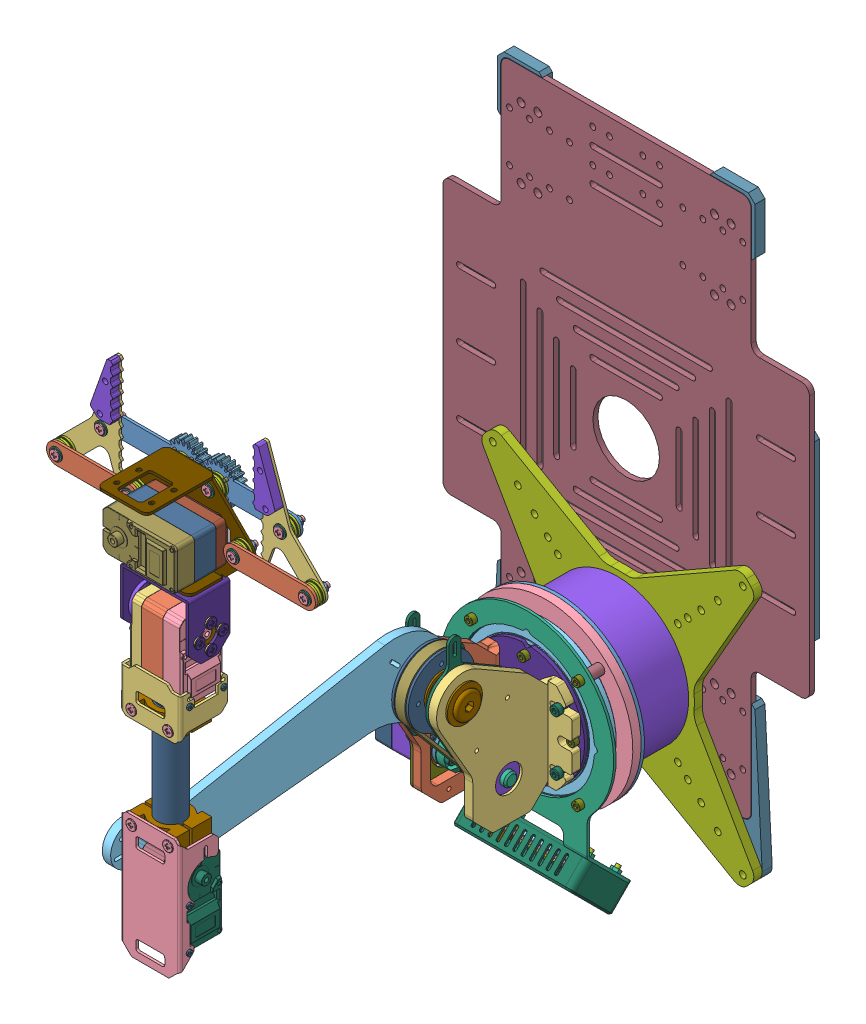
SolidWorks assembly RoArm-M1 STEP, configuration Default. Lengths in mm. (continued)
Components (placement in the parent): (continued)
- RoArm-M1 STEP(2)^RoArm-M1 STEP-1: RoArm-M1 STEP(2)^RoArm-M1 STEP [Default] at origin size (176.32 372.07 316.7) (virtual) (continued)
  - Servo Driver with ESP32^RoArm-M1 STEP(2)_RoArm-M1 STEP-1: Servo Driver with ESP32^RoArm-M1 STEP(2)_RoArm-M1 STEP [Default] at (-32.5 -89.0448 39.0323) x (1 0 0) z (0 -0.707107 0.707107) size (65.89 30.51 11.2) (virtual) (continued)
    - C12^Servo Driver with ESP32_RoArm-M1 STEP(2)_RoArm-M1 STEP-1: C12^Servo Driver with ESP32_RoArm-M1 STEP(2)_RoArm-M1 STEP [Default] at origin size (0.85 1.65 0.46) (virtual) (continued)
      - 490325008_24^C12_Servo Driver with ESP32_RoArm-M1 STEP(2)_RoArm-M1 STEP-1: 490325008_24^C12_Servo Driver with ESP32_RoArm-M1 STEP(2)_RoArm-M1 STEP [Default] at (45.7759 19.8899 -0.8715) size (0.85 0.28 0.46) (virtual) (continued)
        - Extruded (2)^490325008_24_C12_Servo Driver with ESP32_RoArm-M1 STEP(2)_RoArm-M1 STEP-1: Extruded (2)^490325008_24_C12_Servo Driver with ESP32_RoArm-M1 STEP(2)_RoArm-M1 STEP [Default] at origin size (0.85 0.28 0.46) (virtual)
      - 490325008_25^C12_Servo Driver with ESP32_RoArm-M1 STEP(2)_RoArm-M1 STEP-1: 490325008_25^C12_Servo Driver with ESP32_RoArm-M1 STEP(2)_RoArm-M1 STEP [Default] at (45.7759 21.2615 -0.8715) size (0.85 0.28 0.46) (virtual)
        - Extruded (2)^490325008_25_C12_Servo Driver with ESP32_RoArm-M1 STEP(2)_RoArm-M1 STEP-1: Extruded (2)^490325008_25_C12_Servo Driver with ESP32_RoArm-M1 STEP(2)_RoArm-M1 STEP [Default] at origin size (0.85 0.28 0.46) (virtual)
    - C13^Servo Driver with ESP32_RoArm-M1 STEP(2)_RoArm-M1 STEP-1: C13^Servo Driver with ESP32_RoArm-M1 STEP(2)_RoArm-M1 STEP [Default] at origin size (0.85 1.65 0.46) (virtual)
      - 490325136_13^C13_Servo Driver with ESP32_RoArm-M1 STEP(2)_RoArm-M1 STEP-1: 490325136_13^C13_Servo Driver with ESP32_RoArm-M1 STEP(2)_RoArm-M1 STEP [Default] at (44.2999 20.558 -0.8615) size (0.8 1.5 0.42) (virtual)
        - Extruded (3)^490325136_13_C13_Servo Driver with ESP32_RoArm-M1 STEP(2)_RoArm-M1 STEP-1: Extruded (3)^490325136_13_C13_Servo Driver with ESP32_RoArm-M1 STEP(2)_RoArm-M1 STEP [Default] at origin size (0.8 1.5 0.42) (virtual)
      - 490325008_26^C13_Servo Driver with ESP32_RoArm-M1 STEP(2)_RoArm-M1 STEP-1: 490325008_26^C13_Servo Driver with ESP32_RoArm-M1 STEP(2)_RoArm-M1 STEP [Default] at (44.2999 19.8721 -0.8715) size (0.85 0.28 0.46) (virtual)
        - Extruded (2)^490325008_26_C13_Servo Driver with ESP32_RoArm-M1 STEP(2)_RoArm-M1 STEP-1: Extruded (2)^490325008_26_C13_Servo Driver with ESP32_RoArm-M1 STEP(2)_RoArm-M1 STEP [Default] at origin size (0.85 0.28 0.46) (virtual)
      - 490325008_27^C13_Servo Driver with ESP32_RoArm-M1 STEP(2)_RoArm-M1 STEP-1: 490325008_27^C13_Servo Driver with ESP32_RoArm-M1 STEP(2)_RoArm-M1 STEP [Default] at (44.2999 21.2437 -0.8715) size (0.85 0.28 0.46) (virtual)
        - Extruded (2)^490325008_27_C13_Servo Driver with ESP32_RoArm-M1 STEP(2)_RoArm-M1 STEP-1: Extruded (2)^490325008_27_C13_Servo Driver with ESP32_RoArm-M1 STEP(2)_RoArm-M1 STEP [Default] at origin size (0.85 0.28 0.46) (virtual)
    - C15^Servo Driver with ESP32_RoArm-M1 STEP(2)_RoArm-M1 STEP-1: C15^Servo Driver with ESP32_RoArm-M1 STEP(2)_RoArm-M1 STEP [Default] at origin size (1.65 0.85 0.46) (virtual)
      - 490324752_26^C15_Servo Driver with ESP32_RoArm-M1 STEP(2)_RoArm-M1 STEP-1: 490324752_26^C15_Servo Driver with ESP32_RoArm-M1 STEP(2)_RoArm-M1 STEP [Default] at (52.9512 19.6079 -0.8615) size (1.5 0.8 0.42) (virtual)
        - Extruded (7)^490324752_26_C15_Servo Driver with ESP32_RoArm-M1 STEP(2)_RoArm-M1 STEP-1: Extruded (7)^490324752_26_C15_Servo Driver with ESP32_RoArm-M1 STEP(2)_RoArm-M1 STEP [Default] at origin size (1.5 0.8 0.42) (virtual)
      - 490324624_52^C15_Servo Driver with ESP32_RoArm-M1 STEP(2)_RoArm-M1 STEP-1: 490324624_52^C15_Servo Driver with ESP32_RoArm-M1 STEP(2)_RoArm-M1 STEP [Default] at (53.637 19.6079 -0.8715) size (0.28 0.85 0.46) (virtual)
        - Extruded (6)^490324624_52_C15_Servo Driver with ESP32_RoArm-M1 STEP(2)_RoArm-M1 STEP-1: Extruded (6)^490324624_52_C15_Servo Driver with ESP32_RoArm-M1 STEP(2)_RoArm-M1 STEP [Default] at origin size (0.28 0.85 0.46) (virtual)
      - 490324624_53^C15_Servo Driver with ESP32_RoArm-M1 STEP(2)_RoArm-M1 STEP-1: 490324624_53^C15_Servo Driver with ESP32_RoArm-M1 STEP(2)_RoArm-M1 STEP [Default] at (52.2655 19.6079 -0.8715) size (0.28 0.85 0.46) (virtual)
        - Extruded (6)^490324624_53_C15_Servo Driver with ESP32_RoArm-M1 STEP(2)_RoArm-M1 STEP-1: Extruded (6)^490324624_53_C15_Servo Driver with ESP32_RoArm-M1 STEP(2)_RoArm-M1 STEP [Default] at origin size (0.28 0.85 0.46) (virtual)
    - CN1^Servo Driver with ESP32_RoArm-M1 STEP(2)_RoArm-M1 STEP-1: CN1^Servo Driver with ESP32_RoArm-M1 STEP(2)_RoArm-M1 STEP [Default] at origin size (11.53 9.47 7.3) (virtual)
      - 731906128^CN1_Servo Driver with ESP32_RoArm-M1 STEP(2)_RoArm-M1 STEP-1: 731906128^CN1_Servo Driver with ESP32_RoArm-M1 STEP(2)_RoArm-M1 STEP [Default] at (4.8803 15.0759 0) size (11.53 9.47 7.3) (virtual)
        - Extruded (23)^731906128_CN1_Servo Driver with ESP32_RoArm-M1 STEP(2)_RoArm-M1 STEP-1: Extruded (23)^731906128_CN1_Servo Driver with ESP32_RoArm-M1 STEP(2)_RoArm-M1 STEP [Default] at origin size (11.53 9.47 7.3) (virtual)
    - L1(2)^Servo Driver with ESP32_RoArm-M1 STEP(2)_RoArm-M1 STEP-1: L1(2)^Servo Driver with ESP32_RoArm-M1 STEP(2)_RoArm-M1 STEP [Default] at origin size (5 5 2) (virtual)
      - 731906000^L1(2)_Servo Driver with ESP32_RoArm-M1 STEP(2)_RoArm-M1 STEP-1: 731906000^L1(2)_Servo Driver with ESP32_RoArm-M1 STEP(2)_RoArm-M1 STEP [Default] at (27.2498 4.0078 0) size (5 5 2) (virtual)
        - Extruded (24)^731906000_L1(2)_Servo Driver with ESP32_RoArm-M1 STEP(2)_RoArm-M1 STEP-1: Extruded (24)^731906000_L1(2)_Servo Driver with ESP32_RoArm-M1 STEP(2)_RoArm-M1 STEP [Default] at origin size (5 5 2) (virtual)
    - L2(2)^Servo Driver with ESP32_RoArm-M1 STEP(2)_RoArm-M1 STEP-1: L2(2)^Servo Driver with ESP32_RoArm-M1 STEP(2)_RoArm-M1 STEP [Default] at origin size (5 5 2) (virtual)
      - 731906000_1^L2(2)_Servo Driver with ESP32_RoArm-M1 STEP(2)_RoArm-M1 STEP-1: 731906000_1^L2(2)_Servo Driver with ESP32_RoArm-M1 STEP(2)_RoArm-M1 STEP [Default] at (35.2498 4.0078 0) size (5 5 2) (virtual)
        - Extruded (24)^731906000_1_L2(2)_Servo Driver with ESP32_RoArm-M1 STEP(2)_RoArm-M1 STEP-1: Extruded (24)^731906000_1_L2(2)_Servo Driver with ESP32_RoArm-M1 STEP(2)_RoArm-M1 STEP [Default] at origin size (5 5 2) (virtual)
    - R1^Servo Driver with ESP32_RoArm-M1 STEP(2)_RoArm-M1 STEP-1: R1^Servo Driver with ESP32_RoArm-M1 STEP(2)_RoArm-M1 STEP [Default] at origin size (1.65 0.85 0.46) (virtual)
      - 490324752_27^R1_Servo Driver with ESP32_RoArm-M1 STEP(2)_RoArm-M1 STEP-1: 490324752_27^R1_Servo Driver with ESP32_RoArm-M1 STEP(2)_RoArm-M1 STEP [Default] at (32.4997 10.6578 0.025) size (1.5 0.8 0.42) (virtual)
        - Extruded (7)^490324752_27_R1_Servo Driver with ESP32_RoArm-M1 STEP(2)_RoArm-M1 STEP-1: Extruded (7)^490324752_27_R1_Servo Driver with ESP32_RoArm-M1 STEP(2)_RoArm-M1 STEP [Default] at origin size (1.5 0.8 0.42) (virtual)
      - 490324624_54^R1_Servo Driver with ESP32_RoArm-M1 STEP(2)_RoArm-M1 STEP-1: 490324624_54^R1_Servo Driver with ESP32_RoArm-M1 STEP(2)_RoArm-M1 STEP [Default] at (33.1855 10.6578 0.001) size (0.28 0.85 0.46) (virtual)
        - Extruded (6)^490324624_54_R1_Servo Driver with ESP32_RoArm-M1 STEP(2)_RoArm-M1 STEP-1: Extruded (6)^490324624_54_R1_Servo Driver with ESP32_RoArm-M1 STEP(2)_RoArm-M1 STEP [Default] at origin size (0.28 0.85 0.46) (virtual)
      - 490324624_55^R1_Servo Driver with ESP32_RoArm-M1 STEP(2)_RoArm-M1 STEP-1: 490324624_55^R1_Servo Driver with ESP32_RoArm-M1 STEP(2)_RoArm-M1 STEP [Default] at (31.814 10.6578 0.001) size (0.28 0.85 0.46) (virtual)
        - Extruded (6)^490324624_55_R1_Servo Driver with ESP32_RoArm-M1 STEP(2)_RoArm-M1 STEP-1: Extruded (6)^490324624_55_R1_Servo Driver with ESP32_RoArm-M1 STEP(2)_RoArm-M1 STEP [Default] at origin size (0.28 0.85 0.46) (virtual)
    - R2^Servo Driver with ESP32_RoArm-M1 STEP(2)_RoArm-M1 STEP-1: R2^Servo Driver with ESP32_RoArm-M1 STEP(2)_RoArm-M1 STEP [Default] at origin size (1.65 0.85 0.46) (virtual)
      - 490324752_28^R2_Servo Driver with ESP32_RoArm-M1 STEP(2)_RoArm-M1 STEP-1: 490324752_28^R2_Servo Driver with ESP32_RoArm-M1 STEP(2)_RoArm-M1 STEP [Default] at (32.4997 12.1078 0.025) size (1.5 0.8 0.42) (virtual)
        - Extruded (7)^490324752_28_R2_Servo Driver with ESP32_RoArm-M1 STEP(2)_RoArm-M1 STEP-1: Extruded (7)^490324752_28_R2_Servo Driver with ESP32_RoArm-M1 STEP(2)_RoArm-M1 STEP [Default] at origin size (1.5 0.8 0.42) (virtual)
      - 490324624_56^R2_Servo Driver with ESP32_RoArm-M1 STEP(2)_RoArm-M1 STEP-1: 490324624_56^R2_Servo Driver with ESP32_RoArm-M1 STEP(2)_RoArm-M1 STEP [Default] at (33.1855 12.1078 0.001) size (0.28 0.85 0.46) (virtual)
        - Extruded (6)^490324624_56_R2_Servo Driver with ESP32_RoArm-M1 STEP(2)_RoArm-M1 STEP-1: Extruded (6)^490324624_56_R2_Servo Driver with ESP32_RoArm-M1 STEP(2)_RoArm-M1 STEP [Default] at origin size (0.28 0.85 0.46) (virtual)
      - 490324624_57^R2_Servo Driver with ESP32_RoArm-M1 STEP(2)_RoArm-M1 STEP-1: 490324624_57^R2_Servo Driver with ESP32_RoArm-M1 STEP(2)_RoArm-M1 STEP [Default] at (31.814 12.1078 0.001) size (0.28 0.85 0.46) (virtual)
        - Extruded (6)^490324624_57_R2_Servo Driver with ESP32_RoArm-M1 STEP(2)_RoArm-M1 STEP-1: Extruded (6)^490324624_57_R2_Servo Driver with ESP32_RoArm-M1 STEP(2)_RoArm-M1 STEP [Default] at origin size (0.28 0.85 0.46) (virtual)
    - R17^Servo Driver with ESP32_RoArm-M1 STEP(2)_RoArm-M1 STEP-1: R17^Servo Driver with ESP32_RoArm-M1 STEP(2)_RoArm-M1 STEP [Default] at origin size (1.65 0.85 0.46) (virtual)
      - 490324752_29^R17_Servo Driver with ESP32_RoArm-M1 STEP(2)_RoArm-M1 STEP-1: 490324752_29^R17_Servo Driver with ESP32_RoArm-M1 STEP(2)_RoArm-M1 STEP [Default] at (52.9512 22.5079 -0.8615) size (1.5 0.8 0.42) (virtual)
        - Extruded (7)^490324752_29_R17_Servo Driver with ESP32_RoArm-M1 STEP(2)_RoArm-M1 STEP-1: Extruded (7)^490324752_29_R17_Servo Driver with ESP32_RoArm-M1 STEP(2)_RoArm-M1 STEP [Default] at origin size (1.5 0.8 0.42) (virtual)
      - 490324624_58^R17_Servo Driver with ESP32_RoArm-M1 STEP(2)_RoArm-M1 STEP-1: 490324624_58^R17_Servo Driver with ESP32_RoArm-M1 STEP(2)_RoArm-M1 STEP [Default] at (53.637 22.5079 -0.8715) size (0.28 0.85 0.46) (virtual)
        - Extruded (6)^490324624_58_R17_Servo Driver with ESP32_RoArm-M1 STEP(2)_RoArm-M1 STEP-1: Extruded (6)^490324624_58_R17_Servo Driver with ESP32_RoArm-M1 STEP(2)_RoArm-M1 STEP [Default] at origin size (0.28 0.85 0.46) (virtual)
      - 490324624_59^R17_Servo Driver with ESP32_RoArm-M1 STEP(2)_RoArm-M1 STEP-1: 490324624_59^R17_Servo Driver with ESP32_RoArm-M1 STEP(2)_RoArm-M1 STEP [Default] at (52.2655 22.5079 -0.8715) size (0.28 0.85 0.46) (virtual)
        - Extruded (6)^490324624_59_R17_Servo Driver with ESP32_RoArm-M1 STEP(2)_RoArm-M1 STEP-1: Extruded (6)^490324624_59_R17_Servo Driver with ESP32_RoArm-M1 STEP(2)_RoArm-M1 STEP [Default] at origin size (0.28 0.85 0.46) (virtual)
    - R4^Servo Driver with ESP32_RoArm-M1 STEP(2)_RoArm-M1 STEP-1: R4^Servo Driver with ESP32_RoArm-M1 STEP(2)_RoArm-M1 STEP [Default] at origin size (0.85 1.65 0.46) (virtual)
      - 490325136_14^R4_Servo Driver with ESP32_RoArm-M1 STEP(2)_RoArm-M1 STEP-1: 490325136_14^R4_Servo Driver with ESP32_RoArm-M1 STEP(2)_RoArm-M1 STEP [Default] at (56.8497 11.8578 -0.8615) size (0.8 1.5 0.42) (virtual)
        - Extruded (3)^490325136_14_R4_Servo Driver with ESP32_RoArm-M1 STEP(2)_RoArm-M1 STEP-1: Extruded (3)^490325136_14_R4_Servo Driver with ESP32_RoArm-M1 STEP(2)_RoArm-M1 STEP [Default] at origin size (0.8 1.5 0.42) (virtual)
      - 490325008_28^R4_Servo Driver with ESP32_RoArm-M1 STEP(2)_RoArm-M1 STEP-1: 490325008_28^R4_Servo Driver with ESP32_RoArm-M1 STEP(2)_RoArm-M1 STEP [Default] at (56.8497 12.5436 -0.8715) size (0.85 0.28 0.46) (virtual)
        - Extruded (2)^490325008_28_R4_Servo Driver with ESP32_RoArm-M1 STEP(2)_RoArm-M1 STEP-1: Extruded (2)^490325008_28_R4_Servo Driver with ESP32_RoArm-M1 STEP(2)_RoArm-M1 STEP [Default] at origin size (0.85 0.28 0.46) (virtual)
      - 490325008_29^R4_Servo Driver with ESP32_RoArm-M1 STEP(2)_RoArm-M1 STEP-1: 490325008_29^R4_Servo Driver with ESP32_RoArm-M1 STEP(2)_RoArm-M1 STEP [Default] at (56.8497 11.172 -0.8715) size (0.85 0.28 0.46) (virtual)
        - Extruded (2)^490325008_29_R4_Servo Driver with ESP32_RoArm-M1 STEP(2)_RoArm-M1 STEP-1: Extruded (2)^490325008_29_R4_Servo Driver with ESP32_RoArm-M1 STEP(2)_RoArm-M1 STEP [Default] at origin size (0.85 0.28 0.46) (virtual)
    - R5^Servo Driver with ESP32_RoArm-M1 STEP(2)_RoArm-M1 STEP-1: R5^Servo Driver with ESP32_RoArm-M1 STEP(2)_RoArm-M1 STEP [Default] at origin size (0.85 1.65 0.46) (virtual)
      - 490325136_15^R5_Servo Driver with ESP32_RoArm-M1 STEP(2)_RoArm-M1 STEP-1: 490325136_15^R5_Servo Driver with ESP32_RoArm-M1 STEP(2)_RoArm-M1 STEP [Default] at (56.8499 18.158 -0.8615) size (0.8 1.5 0.42) (virtual)
        - Extruded (3)^490325136_15_R5_Servo Driver with ESP32_RoArm-M1 STEP(2)_RoArm-M1 STEP-1: Extruded (3)^490325136_15_R5_Servo Driver with ESP32_RoArm-M1 STEP(2)_RoArm-M1 STEP [Default] at origin size (0.8 1.5 0.42) (virtual)
      - 490325008_30^R5_Servo Driver with ESP32_RoArm-M1 STEP(2)_RoArm-M1 STEP-1: 490325008_30^R5_Servo Driver with ESP32_RoArm-M1 STEP(2)_RoArm-M1 STEP [Default] at (56.8499 17.4721 -0.8715) size (0.85 0.28 0.46) (virtual)
        - Extruded (2)^490325008_30_R5_Servo Driver with ESP32_RoArm-M1 STEP(2)_RoArm-M1 STEP-1: Extruded (2)^490325008_30_R5_Servo Driver with ESP32_RoArm-M1 STEP(2)_RoArm-M1 STEP [Default] at origin size (0.85 0.28 0.46) (virtual)
      - 490325008_31^R5_Servo Driver with ESP32_RoArm-M1 STEP(2)_RoArm-M1 STEP-1: 490325008_31^R5_Servo Driver with ESP32_RoArm-M1 STEP(2)_RoArm-M1 STEP [Default] at (56.8499 18.8437 -0.8715) size (0.85 0.28 0.46) (virtual)
        - Extruded (2)^490325008_31_R5_Servo Driver with ESP32_RoArm-M1 STEP(2)_RoArm-M1 STEP-1: Extruded (2)^490325008_31_R5_Servo Driver with ESP32_RoArm-M1 STEP(2)_RoArm-M1 STEP [Default] at origin size (0.85 0.28 0.46) (virtual)
    - Type_C1^Servo Driver with ESP32_RoArm-M1 STEP(2)_RoArm-M1 STEP-1: Type_C1^Servo Driver with ESP32_RoArm-M1 STEP(2)_RoArm-M1 STEP [Default] at origin size (9.58 7.71 4.16) (virtual)
      - 698b116-264-211^Type_C1_Servo Driver with ESP32_RoArm-M1 STEP(2)_RoArm-M1 STEP-1: 698b116-264-211^Type_C1_Servo Driver with ESP32_RoArm-M1 STEP(2)_RoArm-M1 STEP [Default] at (36.2227 -4.8299 -11.5) x (1 0 0) z (0 -1 0) size (9.58 4.16 7.71) (virtual)
        - SOLID^698b116-264-211_Type_C1_Servo Driver with ESP32_RoArm-M1 STEP(2)_RoArm-M1 STEP-1: SOLID^698b116-264-211_Type_C1_Servo Driver with ESP32_RoArm-M1 STEP(2)_RoArm-M1 STEP [Default] at origin size (8.34 3.56 7.05) (virtual)
        - SOLID (1)^698b116-264-211_Type_C1_Servo Driver with ESP32_RoArm-M1 STEP(2)_RoArm-M1 STEP-1: SOLID (1)^698b116-264-211_Type_C1_Servo Driver with ESP32_RoArm-M1 STEP(2)_RoArm-M1 STEP [Default] at origin size (0.26 1.45 0.87) (virtual)
        - SOLID (2)^698b116-264-211_Type_C1_Servo Driver with ESP32_RoArm-M1 STEP(2)_RoArm-M1 STEP-1: SOLID (2)^698b116-264-211_Type_C1_Servo Driver with ESP32_RoArm-M1 STEP(2)_RoArm-M1 STEP [Default] at origin size (0.26 1.45 0.87) (virtual)
        - SOLID (3)^698b116-264-211_Type_C1_Servo Driver with ESP32_RoArm-M1 STEP(2)_RoArm-M1 STEP-1: SOLID (3)^698b116-264-211_Type_C1_Servo Driver with ESP32_RoArm-M1 STEP(2)_RoArm-M1 STEP [Default] at origin size (0.25 1.45 0.87) (virtual)
        - SOLID (4)^698b116-264-211_Type_C1_Servo Driver with ESP32_RoArm-M1 STEP(2)_RoArm-M1 STEP-1: SOLID (4)^698b116-264-211_Type_C1_Servo Driver with ESP32_RoArm-M1 STEP(2)_RoArm-M1 STEP [Default] at origin size (0.25 1.45 0.87) (virtual)
        - SOLID (5)^698b116-264-211_Type_C1_Servo Driver with ESP32_RoArm-M1 STEP(2)_RoArm-M1 STEP-1: SOLID (5)^698b116-264-211_Type_C1_Servo Driver with ESP32_RoArm-M1 STEP(2)_RoArm-M1 STEP [Default] at origin size (0.25 2.03 6.58) (virtual)
        - SOLID (6)^698b116-264-211_Type_C1_Servo Driver with ESP32_RoArm-M1 STEP(2)_RoArm-M1 STEP-1: SOLID (6)^698b116-264-211_Type_C1_Servo Driver with ESP32_RoArm-M1 STEP(2)_RoArm-M1 STEP [Default] at origin size (0.25 2.03 6.58) (virtual)
        - SOLID (7)^698b116-264-211_Type_C1_Servo Driver with ESP32_RoArm-M1 STEP(2)_RoArm-M1 STEP-1: SOLID (7)^698b116-264-211_Type_C1_Servo Driver with ESP32_RoArm-M1 STEP(2)_RoArm-M1 STEP [Default] at origin size (0.25 1.57 6.58) (virtual)
        - SOLID (8)^698b116-264-211_Type_C1_Servo Driver with ESP32_RoArm-M1 STEP(2)_RoArm-M1 STEP-1: SOLID (8)^698b116-264-211_Type_C1_Servo Driver with ESP32_RoArm-M1 STEP(2)_RoArm-M1 STEP [Default] at origin size (0.25 1.57 6.58) (virtual)
        - SOLID (9)^698b116-264-211_Type_C1_Servo Driver with ESP32_RoArm-M1 STEP(2)_RoArm-M1 STEP-1: SOLID (9)^698b116-264-211_Type_C1_Servo Driver with ESP32_RoArm-M1 STEP(2)_RoArm-M1 STEP [Default] at origin size (0.25 0.24 5.71) (virtual)
        - SOLID (10)^698b116-264-211_Type_C1_Servo Driver with ESP32_RoArm-M1 STEP(2)_RoArm-M1 STEP-1: SOLID (10)^698b116-264-211_Type_C1_Servo Driver with ESP32_RoArm-M1 STEP(2)_RoArm-M1 STEP [Default] at origin size (0.25 0.24 5.71) (virtual)
        - SOLID (11)^698b116-264-211_Type_C1_Servo Driver with ESP32_RoArm-M1 STEP(2)_RoArm-M1 STEP-1: SOLID (11)^698b116-264-211_Type_C1_Servo Driver with ESP32_RoArm-M1 STEP(2)_RoArm-M1 STEP [Default] at origin size (0.85 1.57 7.13) (virtual)
        - SOLID (12)^698b116-264-211_Type_C1_Servo Driver with ESP32_RoArm-M1 STEP(2)_RoArm-M1 STEP-1: SOLID (12)^698b116-264-211_Type_C1_Servo Driver with ESP32_RoArm-M1 STEP(2)_RoArm-M1 STEP [Default] at origin size (0.35 2.03 6.78) (virtual)
        - SOLID (13)^698b116-264-211_Type_C1_Servo Driver with ESP32_RoArm-M1 STEP(2)_RoArm-M1 STEP-1: SOLID (13)^698b116-264-211_Type_C1_Servo Driver with ESP32_RoArm-M1 STEP(2)_RoArm-M1 STEP [Default] at origin size (0.35 0.24 5.91) (virtual)
        - SOLID (14)^698b116-264-211_Type_C1_Servo Driver with ESP32_RoArm-M1 STEP(2)_RoArm-M1 STEP-1: SOLID (14)^698b116-264-211_Type_C1_Servo Driver with ESP32_RoArm-M1 STEP(2)_RoArm-M1 STEP [Default] at origin size (0.35 2.03 6.78) (virtual)
        - SOLID (15)^698b116-264-211_Type_C1_Servo Driver with ESP32_RoArm-M1 STEP(2)_RoArm-M1 STEP-1: SOLID (15)^698b116-264-211_Type_C1_Servo Driver with ESP32_RoArm-M1 STEP(2)_RoArm-M1 STEP [Default] at origin size (0.35 0.24 5.91) (virtual)
        - SOLID (16)^698b116-264-211_Type_C1_Servo Driver with ESP32_RoArm-M1 STEP(2)_RoArm-M1 STEP-1: SOLID (16)^698b116-264-211_Type_C1_Servo Driver with ESP32_RoArm-M1 STEP(2)_RoArm-M1 STEP [Default] at origin size (0.85 1.57 7.13) (virtual)
        - SOLID (17)^698b116-264-211_Type_C1_Servo Driver with ESP32_RoArm-M1 STEP(2)_RoArm-M1 STEP-1: SOLID (17)^698b116-264-211_Type_C1_Servo Driver with ESP32_RoArm-M1 STEP(2)_RoArm-M1 STEP [Default] at origin size (0.25 0.24 4.21) (virtual)
        - SOLID (18)^698b116-264-211_Type_C1_Servo Driver with ESP32_RoArm-M1 STEP(2)_RoArm-M1 STEP-1: SOLID (18)^698b116-264-211_Type_C1_Servo Driver with ESP32_RoArm-M1 STEP(2)_RoArm-M1 STEP [Default] at origin size (0.25 0.24 4.21) (virtual)
        - SOLID (19)^698b116-264-211_Type_C1_Servo Driver with ESP32_RoArm-M1 STEP(2)_RoArm-M1 STEP-1: SOLID (19)^698b116-264-211_Type_C1_Servo Driver with ESP32_RoArm-M1 STEP(2)_RoArm-M1 STEP [Default] at origin size (1.11 2.03 7.13) (virtual)
        - SOLID (20)^698b116-264-211_Type_C1_Servo Driver with ESP32_RoArm-M1 STEP(2)_RoArm-M1 STEP-1: SOLID (20)^698b116-264-211_Type_C1_Servo Driver with ESP32_RoArm-M1 STEP(2)_RoArm-M1 STEP [Default] at origin size (1.12 2.03 7.13) (virtual)
        - SOLID (21)^698b116-264-211_Type_C1_Servo Driver with ESP32_RoArm-M1 STEP(2)_RoArm-M1 STEP-1: SOLID (21)^698b116-264-211_Type_C1_Servo Driver with ESP32_RoArm-M1 STEP(2)_RoArm-M1 STEP [Default] at origin size (9.58 4.16 7.53) (virtual)
    - U1^Servo Driver with ESP32_RoArm-M1 STEP(2)_RoArm-M1 STEP-1: U1^Servo Driver with ESP32_RoArm-M1 STEP(2)_RoArm-M1 STEP [Default] at origin size (5 5 0.89) (virtual)
      - 490333456^U1_Servo Driver with ESP32_RoArm-M1 STEP(2)_RoArm-M1 STEP-1: 490333456^U1_Servo Driver with ESP32_RoArm-M1 STEP(2)_RoArm-M1 STEP [Default] at (37.5114 11.6619 0.01) size (5 5 0.89) (virtual)
        - Extruded (25)^490333456_U1_Servo Driver with ESP32_RoArm-M1 STEP(2)_RoArm-M1 STEP-1: Extruded (25)^490333456_U1_Servo Driver with ESP32_RoArm-M1 STEP(2)_RoArm-M1 STEP [Default] at origin size (5 5 0.89) (virtual)
    - D3^Servo Driver with ESP32_RoArm-M1 STEP(2)_RoArm-M1 STEP-1: D3^Servo Driver with ESP32_RoArm-M1 STEP(2)_RoArm-M1 STEP [Default] at origin size (4.1 1.84 1.3) (virtual)
      - 490329488_1^D3_Servo Driver with ESP32_RoArm-M1 STEP(2)_RoArm-M1 STEP-1: 490329488_1^D3_Servo Driver with ESP32_RoArm-M1 STEP(2)_RoArm-M1 STEP [Default] at (50.5997 11.6878 0.2032) size (4.1 1.84 1.3) (virtual)
        - Extruded (19)^490329488_1_D3_Servo Driver with ESP32_RoArm-M1 STEP(2)_RoArm-M1 STEP-1: Extruded (19)^490329488_1_D3_Servo Driver with ESP32_RoArm-M1 STEP(2)_RoArm-M1 STEP [Default] at origin size (4.1 1.84 1.3) (virtual)
    - L4(2)^Servo Driver with ESP32_RoArm-M1 STEP(2)_RoArm-M1 STEP-1: L4(2)^Servo Driver with ESP32_RoArm-M1 STEP(2)_RoArm-M1 STEP [Default] at origin size (1 2.05 0.51) (virtual)
      - 731907280^L4(2)_Servo Driver with ESP32_RoArm-M1 STEP(2)_RoArm-M1 STEP-1: 731907280^L4(2)_Servo Driver with ESP32_RoArm-M1 STEP(2)_RoArm-M1 STEP [Default] at (45.7998 3.6149 0.508) size (0.91 0.76 0) (virtual)
        - Extruded (26)^731907280_L4(2)_Servo Driver with ESP32_RoArm-M1 STEP(2)_RoArm-M1 STEP-1: Extruded (26)^731907280_L4(2)_Servo Driver with ESP32_RoArm-M1 STEP(2)_RoArm-M1 STEP [Default] at origin size (0.91 0.76 0) (virtual)
      - 731906896^L4(2)_Servo Driver with ESP32_RoArm-M1 STEP(2)_RoArm-M1 STEP-1: 731906896^L4(2)_Servo Driver with ESP32_RoArm-M1 STEP(2)_RoArm-M1 STEP [Default] at (45.7998 3.5829 0.0254) size (0.9 1.75 0.48) (virtual)
        - Extruded (27)^731906896_L4(2)_Servo Driver with ESP32_RoArm-M1 STEP(2)_RoArm-M1 STEP-1: Extruded (27)^731906896_L4(2)_Servo Driver with ESP32_RoArm-M1 STEP(2)_RoArm-M1 STEP [Default] at origin size (0.9 1.75 0.48) (virtual)
      - 731906768^L4(2)_Servo Driver with ESP32_RoArm-M1 STEP(2)_RoArm-M1 STEP-1: 731906768^L4(2)_Servo Driver with ESP32_RoArm-M1 STEP(2)_RoArm-M1 STEP [Default] at (45.7998 2.7054 0.001) size (1 0.29 0.51) (virtual)
        - Extruded (28)^731906768_L4(2)_Servo Driver with ESP32_RoArm-M1 STEP(2)_RoArm-M1 STEP-1: Extruded (28)^731906768_L4(2)_Servo Driver with ESP32_RoArm-M1 STEP(2)_RoArm-M1 STEP [Default] at origin size (1 0.29 0.51) (virtual)
      - 731906640^L4(2)_Servo Driver with ESP32_RoArm-M1 STEP(2)_RoArm-M1 STEP-1: 731906640^L4(2)_Servo Driver with ESP32_RoArm-M1 STEP(2)_RoArm-M1 STEP [Default] at (45.7998 4.4924 0.001) size (1 0.23 0.51) (virtual)
        - Extruded (29)^731906640_L4(2)_Servo Driver with ESP32_RoArm-M1 STEP(2)_RoArm-M1 STEP-1: Extruded (29)^731906640_L4(2)_Servo Driver with ESP32_RoArm-M1 STEP(2)_RoArm-M1 STEP [Default] at origin size (1 0.23 0.51) (virtual)
      - 490325008_32^L4(2)_Servo Driver with ESP32_RoArm-M1 STEP(2)_RoArm-M1 STEP-1: 490325008_32^L4(2)_Servo Driver with ESP32_RoArm-M1 STEP(2)_RoArm-M1 STEP [Default] at (45.7998 2.9576 0.001) size (0.85 0.28 0.46) (virtual)
        - Extruded (2)^490325008_32_L4(2)_Servo Driver with ESP32_RoArm-M1 STEP(2)_RoArm-M1 STEP-1: Extruded (2)^490325008_32_L4(2)_Servo Driver with ESP32_RoArm-M1 STEP(2)_RoArm-M1 STEP [Default] at origin size (0.85 0.28 0.46) (virtual)
      - 490325008_33^L4(2)_Servo Driver with ESP32_RoArm-M1 STEP(2)_RoArm-M1 STEP-1: 490325008_33^L4(2)_Servo Driver with ESP32_RoArm-M1 STEP(2)_RoArm-M1 STEP [Default] at (45.7998 4.1817 0.001) size (0.85 0.28 0.46) (virtual)
        - Extruded (2)^490325008_33_L4(2)_Servo Driver with ESP32_RoArm-M1 STEP(2)_RoArm-M1 STEP-1: Extruded (2)^490325008_33_L4(2)_Servo Driver with ESP32_RoArm-M1 STEP(2)_RoArm-M1 STEP [Default] at origin size (0.85 0.28 0.46) (virtual)
    - R21^Servo Driver with ESP32_RoArm-M1 STEP(2)_RoArm-M1 STEP-1: R21^Servo Driver with ESP32_RoArm-M1 STEP(2)_RoArm-M1 STEP [Default] at origin size (0.85 1.65 0.46) (virtual)
      - 490325136_16^R21_Servo Driver with ESP32_RoArm-M1 STEP(2)_RoArm-M1 STEP-1: 490325136_16^R21_Servo Driver with ESP32_RoArm-M1 STEP(2)_RoArm-M1 STEP [Default] at (43.8997 3.508 0.025) size (0.8 1.5 0.42) (virtual)
        - Extruded (3)^490325136_16_R21_Servo Driver with ESP32_RoArm-M1 STEP(2)_RoArm-M1 STEP-1: Extruded (3)^490325136_16_R21_Servo Driver with ESP32_RoArm-M1 STEP(2)_RoArm-M1 STEP [Default] at origin size (0.8 1.5 0.42) (virtual)
      - 490325008_34^R21_Servo Driver with ESP32_RoArm-M1 STEP(2)_RoArm-M1 STEP-1: 490325008_34^R21_Servo Driver with ESP32_RoArm-M1 STEP(2)_RoArm-M1 STEP [Default] at (43.8997 2.8221 0.001) size (0.85 0.28 0.46) (virtual)
        - Extruded (2)^490325008_34_R21_Servo Driver with ESP32_RoArm-M1 STEP(2)_RoArm-M1 STEP-1: Extruded (2)^490325008_34_R21_Servo Driver with ESP32_RoArm-M1 STEP(2)_RoArm-M1 STEP [Default] at origin size (0.85 0.28 0.46) (virtual)
      - 490325008_35^R21_Servo Driver with ESP32_RoArm-M1 STEP(2)_RoArm-M1 STEP-1: 490325008_35^R21_Servo Driver with ESP32_RoArm-M1 STEP(2)_RoArm-M1 STEP [Default] at (43.8997 4.1937 0.001) size (0.85 0.28 0.46) (virtual)
        - Extruded (2)^490325008_35_R21_Servo Driver with ESP32_RoArm-M1 STEP(2)_RoArm-M1 STEP-1: Extruded (2)^490325008_35_R21_Servo Driver with ESP32_RoArm-M1 STEP(2)_RoArm-M1 STEP [Default] at origin size (0.85 0.28 0.46) (virtual)
    - D4^Servo Driver with ESP32_RoArm-M1 STEP(2)_RoArm-M1 STEP-1: D4^Servo Driver with ESP32_RoArm-M1 STEP(2)_RoArm-M1 STEP [Default] at origin size (1.7 4.3 1.7) (virtual)
      - 513897104^D4_Servo Driver with ESP32_RoArm-M1 STEP(2)_RoArm-M1 STEP-1: 513897104^D4_Servo Driver with ESP32_RoArm-M1 STEP(2)_RoArm-M1 STEP [Default] at (9.2496 28.4079 1.3) x (1 0 0) z (0 1 0) size (1.7 1.7 0.2) (virtual)
        - Cylinder^513897104_D4_Servo Driver with ESP32_RoArm-M1 STEP(2)_RoArm-M1 STEP-1: Cylinder^513897104_D4_Servo Driver with ESP32_RoArm-M1 STEP(2)_RoArm-M1 STEP [Default] at origin size (1.7 1.7 0.2) (virtual)
      - 513897224^D4_Servo Driver with ESP32_RoArm-M1 STEP(2)_RoArm-M1 STEP-1: 513897224^D4_Servo Driver with ESP32_RoArm-M1 STEP(2)_RoArm-M1 STEP [Default] at (9.2497 24.5078 1.3) x (1 0 0) z (0 -1 0) size (1.7 1.7 0.2) (virtual)
        - Cylinder (1)^513897224_D4_Servo Driver with ESP32_RoArm-M1 STEP(2)_RoArm-M1 STEP-1: Cylinder (1)^513897224_D4_Servo Driver with ESP32_RoArm-M1 STEP(2)_RoArm-M1 STEP [Default] at origin size (1.7 1.7 0.2) (virtual)
      - 513897344^D4_Servo Driver with ESP32_RoArm-M1 STEP(2)_RoArm-M1 STEP-1: 513897344^D4_Servo Driver with ESP32_RoArm-M1 STEP(2)_RoArm-M1 STEP [Default] at (9.2497 25.7078 1.3) x (1 0 0) z (0 -1 0) size (1.7 1.7 1) (virtual)
        - Cylinder (2)^513897344_D4_Servo Driver with ESP32_RoArm-M1 STEP(2)_RoArm-M1 STEP-1: Cylinder (2)^513897344_D4_Servo Driver with ESP32_RoArm-M1 STEP(2)_RoArm-M1 STEP [Default] at origin size (1.7 1.7 1) (virtual)
      - 513897464^D4_Servo Driver with ESP32_RoArm-M1 STEP(2)_RoArm-M1 STEP-1: 513897464^D4_Servo Driver with ESP32_RoArm-M1 STEP(2)_RoArm-M1 STEP [Default] at (9.2497 28.4578 1.3) x (1 0 0) z (0 -1 0) size (1.6 1.6 4) (virtual)
        - Cylinder (3)^513897464_D4_Servo Driver with ESP32_RoArm-M1 STEP(2)_RoArm-M1 STEP-1: Cylinder (3)^513897464_D4_Servo Driver with ESP32_RoArm-M1 STEP(2)_RoArm-M1 STEP [Default] at origin size (1.6 1.6 4) (virtual)
    - U3^Servo Driver with ESP32_RoArm-M1 STEP(2)_RoArm-M1 STEP-1: U3^Servo Driver with ESP32_RoArm-M1 STEP(2)_RoArm-M1 STEP [Default] at origin size (2.56 2.98 0.7) (virtual)
      - 682615216^U3_Servo Driver with ESP32_RoArm-M1 STEP(2)_RoArm-M1 STEP-1: 682615216^U3_Servo Driver with ESP32_RoArm-M1 STEP(2)_RoArm-M1 STEP [Default] at (17.1658 17.35 -0.5715) size (1.17 0.4 0.16) (virtual)
        - Extruded (30)^682615216_U3_Servo Driver with ESP32_RoArm-M1 STEP(2)_RoArm-M1 STEP-1: Extruded (30)^682615216_U3_Servo Driver with ESP32_RoArm-M1 STEP(2)_RoArm-M1 STEP [Default] at origin size (1.17 0.4 0.16) (virtual)
      - 682615216_1^U3_Servo Driver with ESP32_RoArm-M1 STEP(2)_RoArm-M1 STEP-1: 682615216_1^U3_Servo Driver with ESP32_RoArm-M1 STEP(2)_RoArm-M1 STEP [Default] at (17.1658 16.4102 -0.5715) size (1.17 0.4 0.16) (virtual)
        - Extruded (30)^682615216_1_U3_Servo Driver with ESP32_RoArm-M1 STEP(2)_RoArm-M1 STEP-1: Extruded (30)^682615216_1_U3_Servo Driver with ESP32_RoArm-M1 STEP(2)_RoArm-M1 STEP [Default] at origin size (1.17 0.4 0.16) (virtual)
      - 682615216_2^U3_Servo Driver with ESP32_RoArm-M1 STEP(2)_RoArm-M1 STEP-1: 682615216_2^U3_Servo Driver with ESP32_RoArm-M1 STEP(2)_RoArm-M1 STEP [Default] at (17.1658 15.4704 -0.5715) size (1.17 0.4 0.16) (virtual)
        - Extruded (30)^682615216_2_U3_Servo Driver with ESP32_RoArm-M1 STEP(2)_RoArm-M1 STEP-1: Extruded (30)^682615216_2_U3_Servo Driver with ESP32_RoArm-M1 STEP(2)_RoArm-M1 STEP [Default] at origin size (1.17 0.4 0.16) (virtual)
      - 682615216_3^U3_Servo Driver with ESP32_RoArm-M1 STEP(2)_RoArm-M1 STEP-1: 682615216_3^U3_Servo Driver with ESP32_RoArm-M1 STEP(2)_RoArm-M1 STEP [Default] at (15.7766 15.445 -0.5715) size (1.17 0.4 0.16) (virtual)
        - Extruded (30)^682615216_3_U3_Servo Driver with ESP32_RoArm-M1 STEP(2)_RoArm-M1 STEP-1: Extruded (30)^682615216_3_U3_Servo Driver with ESP32_RoArm-M1 STEP(2)_RoArm-M1 STEP [Default] at origin size (1.17 0.4 0.16) (virtual)
      - 682615216_4^U3_Servo Driver with ESP32_RoArm-M1 STEP(2)_RoArm-M1 STEP-1: 682615216_4^U3_Servo Driver with ESP32_RoArm-M1 STEP(2)_RoArm-M1 STEP [Default] at (15.7766 17.3246 -0.5715) size (1.17 0.4 0.16) (virtual)
        - Extruded (30)^682615216_4_U3_Servo Driver with ESP32_RoArm-M1 STEP(2)_RoArm-M1 STEP-1: Extruded (30)^682615216_4_U3_Servo Driver with ESP32_RoArm-M1 STEP(2)_RoArm-M1 STEP [Default] at origin size (1.17 0.4 0.16) (virtual)
      - 731907152^U3_Servo Driver with ESP32_RoArm-M1 STEP(2)_RoArm-M1 STEP-1: 731907152^U3_Servo Driver with ESP32_RoArm-M1 STEP(2)_RoArm-M1 STEP [Default] at (16.4531 16.4083 -1.1115) size (1.42 2.98 0.65) (virtual)
        - Extruded (31)^731907152_U3_Servo Driver with ESP32_RoArm-M1 STEP(2)_RoArm-M1 STEP-1: Extruded (31)^731907152_U3_Servo Driver with ESP32_RoArm-M1 STEP(2)_RoArm-M1 STEP [Default] at origin size (1.42 2.98 0.65) (virtual)
    - U4^Servo Driver with ESP32_RoArm-M1 STEP(2)_RoArm-M1 STEP-1: U4^Servo Driver with ESP32_RoArm-M1 STEP(2)_RoArm-M1 STEP [Default] at origin size (2.56 2.98 0.7) (virtual)
      - 682615216_5^U4_Servo Driver with ESP32_RoArm-M1 STEP(2)_RoArm-M1 STEP-1: 682615216_5^U4_Servo Driver with ESP32_RoArm-M1 STEP(2)_RoArm-M1 STEP [Default] at (15.2658 21.75 -0.5715) size (1.17 0.4 0.16) (virtual)
        - Extruded (30)^682615216_5_U4_Servo Driver with ESP32_RoArm-M1 STEP(2)_RoArm-M1 STEP-1: Extruded (30)^682615216_5_U4_Servo Driver with ESP32_RoArm-M1 STEP(2)_RoArm-M1 STEP [Default] at origin size (1.17 0.4 0.16) (virtual)
      - 682615216_6^U4_Servo Driver with ESP32_RoArm-M1 STEP(2)_RoArm-M1 STEP-1: 682615216_6^U4_Servo Driver with ESP32_RoArm-M1 STEP(2)_RoArm-M1 STEP [Default] at (15.2658 20.8102 -0.5715) size (1.17 0.4 0.16) (virtual)
        - Extruded (30)^682615216_6_U4_Servo Driver with ESP32_RoArm-M1 STEP(2)_RoArm-M1 STEP-1: Extruded (30)^682615216_6_U4_Servo Driver with ESP32_RoArm-M1 STEP(2)_RoArm-M1 STEP [Default] at origin size (1.17 0.4 0.16) (virtual)
      - 682615216_7^U4_Servo Driver with ESP32_RoArm-M1 STEP(2)_RoArm-M1 STEP-1: 682615216_7^U4_Servo Driver with ESP32_RoArm-M1 STEP(2)_RoArm-M1 STEP [Default] at (15.2658 19.8704 -0.5715) size (1.17 0.4 0.16) (virtual)
        - Extruded (30)^682615216_7_U4_Servo Driver with ESP32_RoArm-M1 STEP(2)_RoArm-M1 STEP-1: Extruded (30)^682615216_7_U4_Servo Driver with ESP32_RoArm-M1 STEP(2)_RoArm-M1 STEP [Default] at origin size (1.17 0.4 0.16) (virtual)
      - 682615216_8^U4_Servo Driver with ESP32_RoArm-M1 STEP(2)_RoArm-M1 STEP-1: 682615216_8^U4_Servo Driver with ESP32_RoArm-M1 STEP(2)_RoArm-M1 STEP [Default] at (13.8766 19.845 -0.5715) size (1.17 0.4 0.16) (virtual)
        - Extruded (30)^682615216_8_U4_Servo Driver with ESP32_RoArm-M1 STEP(2)_RoArm-M1 STEP-1: Extruded (30)^682615216_8_U4_Servo Driver with ESP32_RoArm-M1 STEP(2)_RoArm-M1 STEP [Default] at origin size (1.17 0.4 0.16) (virtual)
      - 682615216_9^U4_Servo Driver with ESP32_RoArm-M1 STEP(2)_RoArm-M1 STEP-1: 682615216_9^U4_Servo Driver with ESP32_RoArm-M1 STEP(2)_RoArm-M1 STEP [Default] at (13.8766 21.7246 -0.5715) size (1.17 0.4 0.16) (virtual)
        - Extruded (30)^682615216_9_U4_Servo Driver with ESP32_RoArm-M1 STEP(2)_RoArm-M1 STEP-1: Extruded (30)^682615216_9_U4_Servo Driver with ESP32_RoArm-M1 STEP(2)_RoArm-M1 STEP [Default] at origin size (1.17 0.4 0.16) (virtual)
      - 731907152_1^U4_Servo Driver with ESP32_RoArm-M1 STEP(2)_RoArm-M1 STEP-1: 731907152_1^U4_Servo Driver with ESP32_RoArm-M1 STEP(2)_RoArm-M1 STEP [Default] at (14.5531 20.8083 -1.1115) size (1.42 2.98 0.65) (virtual)
        - Extruded (31)^731907152_1_U4_Servo Driver with ESP32_RoArm-M1 STEP(2)_RoArm-M1 STEP-1: Extruded (31)^731907152_1_U4_Servo Driver with ESP32_RoArm-M1 STEP(2)_RoArm-M1 STEP [Default] at origin size (1.42 2.98 0.65) (virtual)
    - C24^Servo Driver with ESP32_RoArm-M1 STEP(2)_RoArm-M1 STEP-1: C24^Servo Driver with ESP32_RoArm-M1 STEP(2)_RoArm-M1 STEP [Default] at origin size (1.65 0.85 0.46) (virtual)
      - 490324752_30^C24_Servo Driver with ESP32_RoArm-M1 STEP(2)_RoArm-M1 STEP-1: 490324752_30^C24_Servo Driver with ESP32_RoArm-M1 STEP(2)_RoArm-M1 STEP [Default] at (14.2001 17.2001 0.025) size (1.5 0.8 0.42) (virtual)
        - Extruded (7)^490324752_30_C24_Servo Driver with ESP32_RoArm-M1 STEP(2)_RoArm-M1 STEP-1: Extruded (7)^490324752_30_C24_Servo Driver with ESP32_RoArm-M1 STEP(2)_RoArm-M1 STEP [Default] at origin size (1.5 0.8 0.42) (virtual)
      - 490324624_60^C24_Servo Driver with ESP32_RoArm-M1 STEP(2)_RoArm-M1 STEP-1: 490324624_60^C24_Servo Driver with ESP32_RoArm-M1 STEP(2)_RoArm-M1 STEP [Default] at (13.5143 17.2001 0.001) size (0.28 0.85 0.46) (virtual)
        - Extruded (6)^490324624_60_C24_Servo Driver with ESP32_RoArm-M1 STEP(2)_RoArm-M1 STEP-1: Extruded (6)^490324624_60_C24_Servo Driver with ESP32_RoArm-M1 STEP(2)_RoArm-M1 STEP [Default] at origin size (0.28 0.85 0.46) (virtual)
      - 490324624_61^C24_Servo Driver with ESP32_RoArm-M1 STEP(2)_RoArm-M1 STEP-1: 490324624_61^C24_Servo Driver with ESP32_RoArm-M1 STEP(2)_RoArm-M1 STEP [Default] at (14.8858 17.2001 0.001) size (0.28 0.85 0.46) (virtual)
        - Extruded (6)^490324624_61_C24_Servo Driver with ESP32_RoArm-M1 STEP(2)_RoArm-M1 STEP-1: Extruded (6)^490324624_61_C24_Servo Driver with ESP32_RoArm-M1 STEP(2)_RoArm-M1 STEP [Default] at origin size (0.28 0.85 0.46) (virtual)
    - Board^Servo Driver with ESP32_RoArm-M1 STEP(2)_RoArm-M1 STEP-1: Board^Servo Driver with ESP32_RoArm-M1 STEP(2)_RoArm-M1 STEP [Default] at (0 0 -0.4115) size (65 30.02 1.61) (virtual)
